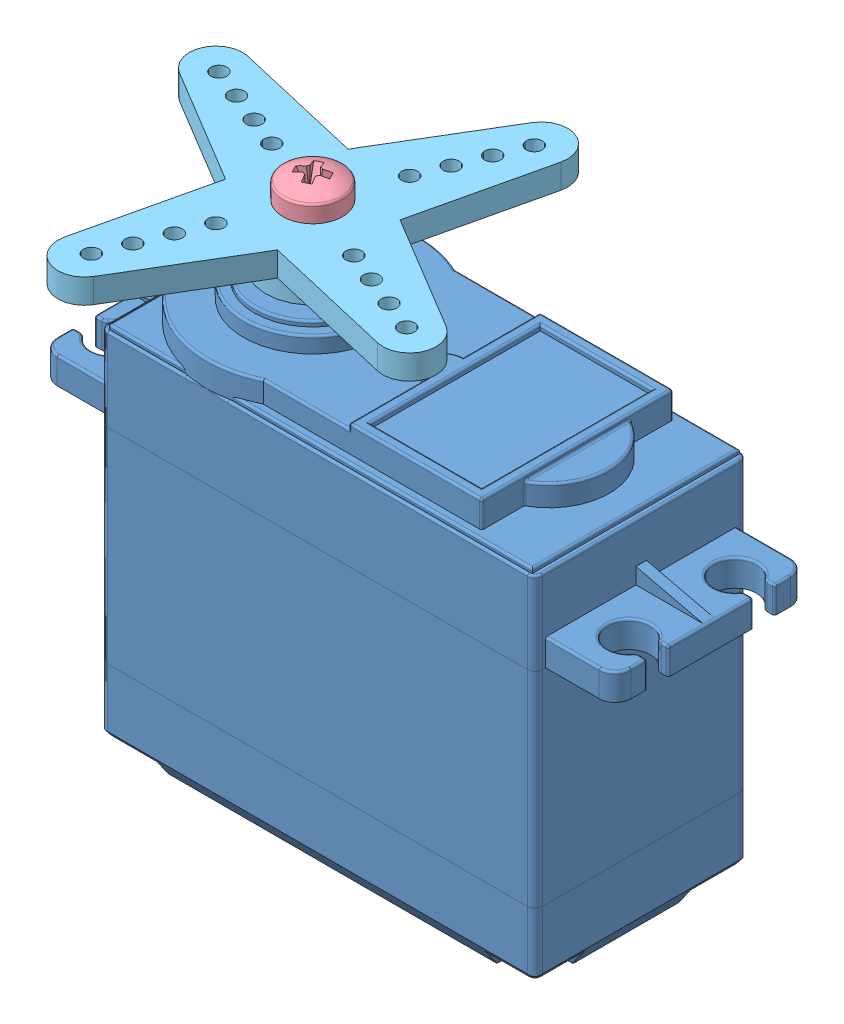
SolidWorks assembly MG996R Servo Motor, configuration Default. Lengths in mm.
Overall size (62.19 47.35 49.48).
14 component instances, 10 part files, 2 mates.
Components (placement in the parent):
- Case-1-1: Case-1 [Default] at origin size (54 39 20)
- Output Shaft-1-1: Output Shaft-1 [Default] at (-10.45 9.35 0) x (0.84541 0 0.534117) z (-0.534117 0 0.84541) size (13.78 15.2 13.78)
- Rubber Wire Cable Sleeve-1-1: Rubber Wire Cable Sleeve-1 [Default] at (-18.2 -12.025 0) size (15.24 5.03 7.75) (hidden)
- Pan Head Cross Screw M1.6-1-1: Pan Head Cross Screw M1.6-1 [Default] at (17.575 12.35 -7.125) x (0 1 0) z (0.499198 0 0.866488) size (32.17 3.2 3.2)
- Pan Head Cross Screw M1.6-1-2: Pan Head Cross Screw M1.6-1 [Default] at (17.575 12.35 7.125) x (0 1 0) z (0.498431 0 0.86693) size (32.17 3.2 3.2)
- Pan Head Cross Screw M1.6-1-3: Pan Head Cross Screw M1.6-1 [Default] at (-17.575 12.35 7.125) x (0 1 0) z (0.509945 0 0.860207) size (32.17 3.2 3.2)
- Pan Head Cross Screw M1.6-1-4: Pan Head Cross Screw M1.6-1 [Default] at (-17.575 12.35 -7.125) x (0 1 0) z (0.500246 0 0.865884) size (32.17 3.2 3.2)
- Servo Horns(2 Horns)-1: Servo Horns(2 Horns) [Default] at (-23.734 -17 33.4052) x (0.994889 0 0.100979) z (-0.100979 0 0.994889) size (38 5.5 12) (hidden)
- Servo Horns(2 Horns)-2: Servo Horns(2 Horns) [Default] at (-10.45 25.7 0) x (-0.366242 0 0.930519) z (0.930519 0 0.366242) size (38 5.5 12) (hidden)
- Pan Head Cross Screw M3-1-1: Pan Head Cross Screw M3-1 [Default] at (-10.45 20.85 0) x (0 -1 0) z (0.893136 0 -0.449786) size (8.51 5.6 5.6)
- Servo Horns(1 Horn)-1: Servo Horns(1 Horn) [Default] at (-24.387 -17 16.7031) x (0.994889 0 0.100979) z (-0.100979 0 0.994889) size (25 5.5 12) (hidden)
- Servo Horns(4 Horns)-1: Servo Horns(4 Horns) [Default] at (-10.45 25.7 0) x (-0.374969 0 0.927037) z (0.927037 0 0.374969) size (38 5.5 38)
- Servo Horns(6 Horns)-1: Servo Horns(6 Horns) [Default] at (-25.9857 -17 59.7933) x (0.994889 0 0.100979) z (-0.100979 0 0.994889) size (32 5.5 28.38) (hidden)
- Servo Horns(Circular Horn)-1: Servo Horns(Circular Horn) [Default] at (8.0165 -17 66.2028) x (0.994889 0 0.100979) z (-0.100979 0 0.994889) size (20 5.5 20) (hidden)
Mates (geometry in assembly coordinates):
- Coincident1: coincident anti-aligned: plane of Pan Head Cross Screw M3-1-1 through (-9.1103 26.85 -0.6747) normal (0 -1 0); plane of Servo Horns(4 Horns)-1 through (-10.45 26.85 0) normal (0 1 0)
- Concentric1: concentric anti-aligned: cone of Output Shaft-1-1 through (-10.45 24.55 0) axis (0 -1 0); cylinder of Servo Horns(4 Horns)-1 through (-10.45 24.55 0) axis (0 1 0) radius 1.5
